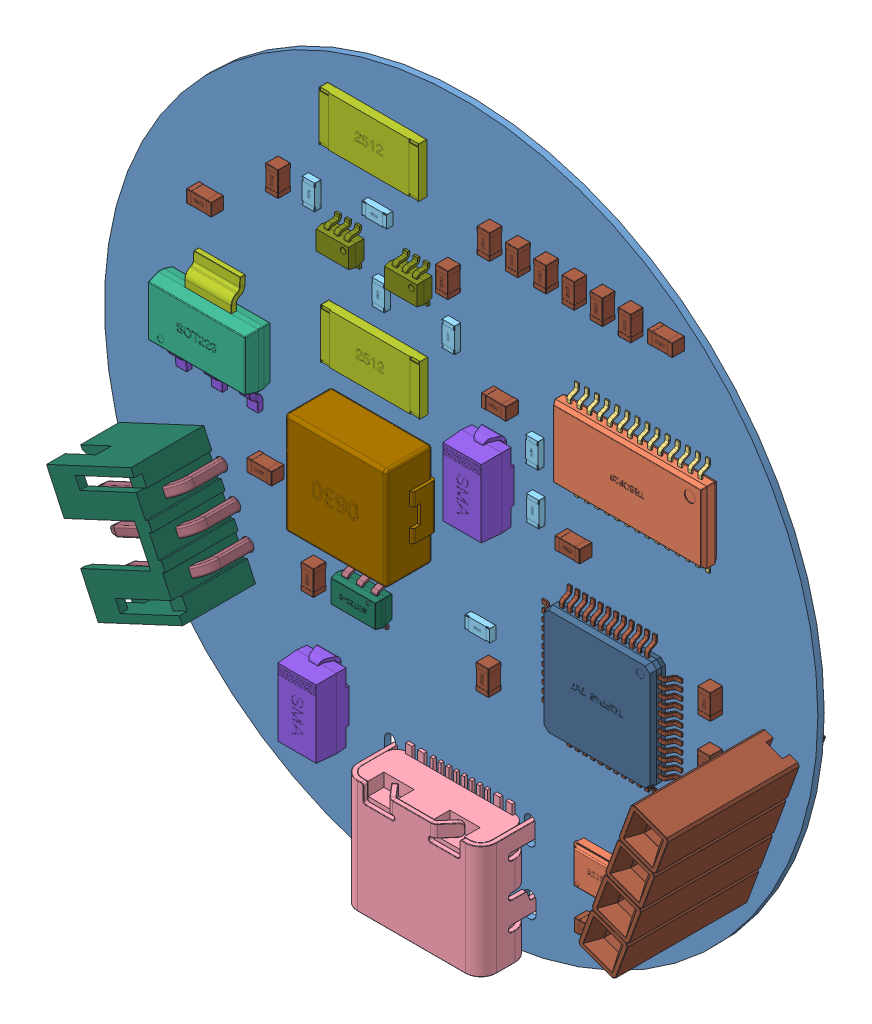
SolidWorks assembly STM32G4_4008_brushless_motor_pcb, configuration 默认. Lengths in mm.
Overall size (46 46 11.81).
338 component instances, 47 part files, 0 mates.
Components (placement in the parent):
- STM32G4_4008_brushless_motor_pcb.step-1: STM32G4_4008_brushless_motor_pcb.step [默认] at origin size (46 46 11.81)
  - Board.step-1: Board.step [默认] at origin size (46 46 0.41)
    - Open CASCADE STEP translator 6.8 1.1.1.step-1: Open CASCADE STEP translator 6.8 1.1.1.step [默认] at (0 0 -0.4115) size (46 46 0.41)
  - X1.step-1: X1.step [默认] at origin size (3.2 2.5 0.72)
    - OSC_3225-4.step-1: OSC_3225-4.step [默认] at (100.5332 55.0164 0) size (3.2 2.5 0.72)
      - OSC_3225-4-0.step-1: OSC_3225-4-0.step [默认] at origin size (3.2 2.5 0.72)
      - LOGO_0.15.step-1: LOGO_0.15.step [默认] at (-0.0166 0.0115 -0.003) size (0.45 0.52 0)
  - USB1.step-1: USB1.step [默认] at origin size (8.94 7.9 4.1)
    - USB_Type-C_A.step-1: USB_Type-C_A.step [默认] at (91.2368 50.7239 0) x (-1 0 0) z (0 0 1) size (8.94 7.9 4.1)
      - USB_Type-C_A-1.step-1: USB_Type-C_A-1.step [默认] at origin size (8.94 7.9 4.1)
      - LOGO_0.5.step-1: LOGO_0.5.step [默认] at (0.0308 -0.1109 0.04) size (1.5 1.73 0.01)
  - U7.step-1: U7.step [默认] at origin size (6.5 7.02 1.67)
    - SOT223.step-1: SOT223.step [默认] at (75.7682 73.3044 0) size (6.5 7.02 1.67)
      - SOT223-2.step-1: SOT223-2.step [默认] at origin size (6.5 3.5 1.6)
      - SOT223___-1.step-1: SOT223___-1.step [默认] at (0 1.75 0.725) size (3 1.76 0.92)
      - SOT223___-2.step-1: SOT223___-2.step [默认] at (2.3 -1.75 0.725) x (-1 0 0) z (0 0 1) size (0.71 1.76 0.92)
      - SOT223___-2.step-2: SOT223___-2.step [默认] at (0 -1.75 0.725) x (-1 0 0) z (0 0 1) size (0.71 1.76 0.92)
      - SOT223___-2.step-3: SOT223___-2.step [默认] at (-2.3 -1.75 0.725) x (-1 0 0) z (0 0 1) size (0.71 1.76 0.92)
      - LOGO_0.25.step-1: LOGO_0.25.step [默认] at origin size (0.75 0.87 0.01)
  - U6.step-1: U6.step [默认] at origin size (9 9 1.05)
    - TQFP48_7x7.step-1: TQFP48_7x7.step [默认] at (100.9904 65.4812 0) x (-1 0 0) z (0 0 1) size (9 9 1.05)
      - TQFP48_7x7______.step-1: TQFP48_7x7______.step [默认] at origin size (7 7 1)
      - _____0.25.step-1: _____0.25.step [默认] at (2.75 -3.5 0.55) x (-1 0 0) z (0 0 1) size (0.25 1 0.6)
      - _____0.25.step-2: _____0.25.step [默认] at (2.25 -3.5 0.55) x (-1 0 0) z (0 0 1) size (0.25 1 0.6)
      - _____0.25.step-3: _____0.25.step [默认] at (1.75 -3.5 0.55) x (-1 0 0) z (0 0 1) size (0.25 1 0.6)
      - _____0.25.step-4: _____0.25.step [默认] at (1.25 -3.5 0.55) x (-1 0 0) z (0 0 1) size (0.25 1 0.6)
      - _____0.25.step-5: _____0.25.step [默认] at (0.75 -3.5 0.55) x (-1 0 0) z (0 0 1) size (0.25 1 0.6)
      - _____0.25.step-6: _____0.25.step [默认] at (0.25 -3.5 0.55) x (-1 0 0) z (0 0 1) size (0.25 1 0.6)
      - _____0.25.step-7: _____0.25.step [默认] at (-0.25 -3.5 0.55) x (-1 0 0) z (0 0 1) size (0.25 1 0.6)
      - _____0.25.step-8: _____0.25.step [默认] at (-0.75 -3.5 0.55) x (-1 0 0) z (0 0 1) size (0.25 1 0.6)
      - _____0.25.step-9: _____0.25.step [默认] at (-1.25 -3.5 0.55) x (-1 0 0) z (0 0 1) size (0.25 1 0.6)
      - _____0.25.step-10: _____0.25.step [默认] at (-1.75 -3.5 0.55) x (-1 0 0) z (0 0 1) size (0.25 1 0.6)
      - _____0.25.step-11: _____0.25.step [默认] at (-2.25 -3.5 0.55) x (-1 0 0) z (0 0 1) size (0.25 1 0.6)
      - _____0.25.step-12: _____0.25.step [默认] at (-2.75 -3.5 0.55) x (-1 0 0) z (0 0 1) size (0.25 1 0.6)
      - _____0.25.step-13: _____0.25.step [默认] at (3.5 2.75 0.55) x (0 -1 0) z (0 0 1) size (0.25 1 0.6)
      - _____0.25.step-14: _____0.25.step [默认] at (-2.75 3.5 0.55) size (0.25 1 0.6)
      - _____0.25.step-15: _____0.25.step [默认] at (-3.5 -2.75 0.55) x (0 1 0) z (0 0 1) size (0.25 1 0.6)
      - _____0.25.step-16: _____0.25.step [默认] at (3.5 2.25 0.55) x (0 -1 0) z (0 0 1) size (0.25 1 0.6)
      - _____0.25.step-17: _____0.25.step [默认] at (-2.25 3.5 0.55) size (0.25 1 0.6)
      - _____0.25.step-18: _____0.25.step [默认] at (-3.5 -2.25 0.55) x (0 1 0) z (0 0 1) size (0.25 1 0.6)
      - _____0.25.step-19: _____0.25.step [默认] at (3.5 1.75 0.55) x (0 -1 0) z (0 0 1) size (0.25 1 0.6)
      - _____0.25.step-20: _____0.25.step [默认] at (-1.75 3.5 0.55) size (0.25 1 0.6)
      - _____0.25.step-21: _____0.25.step [默认] at (-3.5 -1.75 0.55) x (0 1 0) z (0 0 1) size (0.25 1 0.6)
      - _____0.25.step-22: _____0.25.step [默认] at (3.5 1.25 0.55) x (0 -1 0) z (0 0 1) size (0.25 1 0.6)
      - _____0.25.step-23: _____0.25.step [默认] at (-1.25 3.5 0.55) size (0.25 1 0.6)
      - _____0.25.step-24: _____0.25.step [默认] at (-3.5 -1.25 0.55) x (0 1 0) z (0 0 1) size (0.25 1 0.6)
      - _____0.25.step-25: _____0.25.step [默认] at (3.5 0.75 0.55) x (0 -1 0) z (0 0 1) size (0.25 1 0.6)
      - _____0.25.step-26: _____0.25.step [默认] at (-0.75 3.5 0.55) size (0.25 1 0.6)
      - _____0.25.step-27: _____0.25.step [默认] at (-3.5 -0.75 0.55) x (0 1 0) z (0 0 1) size (0.25 1 0.6)
      - _____0.25.step-28: _____0.25.step [默认] at (3.5 0.25 0.55) x (0 -1 0) z (0 0 1) size (0.25 1 0.6)
      - _____0.25.step-29: _____0.25.step [默认] at (-0.25 3.5 0.55) size (0.25 1 0.6)
      - _____0.25.step-30: _____0.25.step [默认] at (-3.5 -0.25 0.55) x (0 1 0) z (0 0 1) size (0.25 1 0.6)
      - _____0.25.step-31: _____0.25.step [默认] at (3.5 -0.25 0.55) x (0 -1 0) z (0 0 1) size (0.25 1 0.6)
      - _____0.25.step-32: _____0.25.step [默认] at (0.25 3.5 0.55) size (0.25 1 0.6)
      - _____0.25.step-33: _____0.25.step [默认] at (-3.5 0.25 0.55) x (0 1 0) z (0 0 1) size (0.25 1 0.6)
      - _____0.25.step-34: _____0.25.step [默认] at (3.5 -0.75 0.55) x (0 -1 0) z (0 0 1) size (0.25 1 0.6)
      - _____0.25.step-35: _____0.25.step [默认] at (0.75 3.5 0.55) size (0.25 1 0.6)
      - _____0.25.step-36: _____0.25.step [默认] at (-3.5 0.75 0.55) x (0 1 0) z (0 0 1) size (0.25 1 0.6)
      - _____0.25.step-37: _____0.25.step [默认] at (3.5 -1.25 0.55) x (0 -1 0) z (0 0 1) size (0.25 1 0.6)
      - _____0.25.step-38: _____0.25.step [默认] at (1.25 3.5 0.55) size (0.25 1 0.6)
      - _____0.25.step-39: _____0.25.step [默认] at (-3.5 1.25 0.55) x (0 1 0) z (0 0 1) size (0.25 1 0.6)
      - _____0.25.step-40: _____0.25.step [默认] at (3.5 -1.75 0.55) x (0 -1 0) z (0 0 1) size (0.25 1 0.6)
      - _____0.25.step-41: _____0.25.step [默认] at (1.75 3.5 0.55) size (0.25 1 0.6)
      - _____0.25.step-42: _____0.25.step [默认] at (-3.5 1.75 0.55) x (0 1 0) z (0 0 1) size (0.25 1 0.6)
      - _____0.25.step-43: _____0.25.step [默认] at (3.5 -2.25 0.55) x (0 -1 0) z (0 0 1) size (0.25 1 0.6)
      - _____0.25.step-44: _____0.25.step [默认] at (2.25 3.5 0.55) size (0.25 1 0.6)
      - _____0.25.step-45: _____0.25.step [默认] at (-3.5 2.25 0.55) x (0 1 0) z (0 0 1) size (0.25 1 0.6)
      - _____0.25.step-46: _____0.25.step [默认] at (3.5 -2.75 0.55) x (0 -1 0) z (0 0 1) size (0.25 1 0.6)
      - _____0.25.step-47: _____0.25.step [默认] at (2.75 3.5 0.55) size (0.25 1 0.6)
      - _____0.25.step-48: _____0.25.step [默认] at (-3.5 2.75 0.55) x (0 1 0) z (0 0 1) size (0.25 1 0.6)
      - LOGO_0.25-3.step-1: LOGO_0.25-3.step [默认] at (0.012 -0.0139 0.045) size (0.75 0.87 0.01)
  - U5.step-1: U5.step [默认] at origin size (3 2.81 1.18)
    - SOT23-6.step-1: SOT23-6.step [默认] at (85.3693 63.043 0) x (-1 0 0) z (0 0 1) size (3 2.81 1.18)
      - SOT23-5and6_____.step-1: SOT23-5and6_____.step [默认] at (-0.95 -0.8 0.675) x (-1 0 0) z (0 0 1) size (0.4 0.6 0.78)
      - SOT23-5and6_____.step-2: SOT23-5and6_____.step [默认] at (0 -0.8 0.675) x (-1 0 0) z (0 0 1) size (0.4 0.6 0.78)
      - SOT23-5and6_____.step-3: SOT23-5and6_____.step [默认] at (0.95 -0.8 0.675) x (-1 0 0) z (0 0 1) size (0.4 0.6 0.78)
      - SOT23-5and6_____.step-4: SOT23-5and6_____.step [默认] at (-0.95 0.8 0.675) size (0.4 0.6 0.78)
      - SOT23-5and6_____.step-5: SOT23-5and6_____.step [默认] at (0.95 0.8 0.675) size (0.4 0.6 0.78)
      - LOGO_0.15-4.step-1: LOGO_0.15-4.step [默认] at (0 -0.0167 0.0485) x (-1 0 0) z (0 0 -1) size (0.45 0.52 0)
      - SOT23-6-5.step-1: SOT23-6-5.step [默认] at origin size (3 1.6 1.1)
      - SOT23-5and6_____.step-6: SOT23-5and6_____.step [默认] at (0 0.8 0.675) size (0.4 0.6 0.78)
  - U4.step-1: U4.step [默认] at origin size (2.2 2.4 1.1)
    - User_Library-SOT363-2.step-1: User_Library-SOT363-2.step [默认] at (83.9827 82.123 0) x (-1 0 0) z (0 0 1) size (2.2 2.4 1.1)
  - U3.step-1: U3.step [默认] at origin size (2.2 2.4 1.1)
    - User_Library-SOT363-2.step-1: User_Library-SOT363-2.step [默认] at (88.3815 82.2404 0) x (-1 0 0) z (0 0 1) size (2.2 2.4 1.1)
  - U2.step-1: U2.step [默认] at origin size (6.01 5 1.9)
    - SOP8.step-1: SOP8.step [默认] at (91.186 70.612 -0.4115) x (-1 0 0) z (0 0 -1) size (6.01 5 1.9)
      - LOGO_0.25-6.step-1: LOGO_0.25-6.step [默认] at (0.0116 0 0.095) x (0 -1 0) z (0 0 -1) size (0.75 0.87 0.01)
      - SOP8_____.step-1: SOP8_____.step [默认] at origin size (3.6 5 1.8)
      - ____1.8_______.step-1: ____1.8_______.step [默认] at (1.8 1.91 1) x (0 1 0) z (0 0 1) size (0.5 1.2 1.1)
      - ____1.8_______.step-2: ____1.8_______.step [默认] at (1.8 0.64 1) x (0 1 0) z (0 0 1) size (0.5 1.2 1.1)
      - ____1.8_______.step-3: ____1.8_______.step [默认] at (1.8 -0.63 1) x (0 1 0) z (0 0 1) size (0.5 1.2 1.1)
      - ____1.8_______.step-4: ____1.8_______.step [默认] at (1.8 -1.9 1) x (0 1 0) z (0 0 1) size (0.5 1.2 1.1)
      - ____1.8_______.step-5: ____1.8_______.step [默认] at (-1.8 1.91 1) x (0 -1 0) z (0 0 1) size (0.5 1.2 1.1)
      - ____1.8_______.step-6: ____1.8_______.step [默认] at (-1.8 0.64 1) x (0 -1 0) z (0 0 1) size (0.5 1.2 1.1)
      - ____1.8_______.step-7: ____1.8_______.step [默认] at (-1.8 -0.63 1) x (0 -1 0) z (0 0 1) size (0.5 1.2 1.1)
      - ____1.8_______.step-8: ____1.8_______.step [默认] at (-1.8 -1.9 1) x (0 -1 0) z (0 0 1) size (0.5 1.2 1.1)
  - U1.step-1: U1.step [默认] at origin size (9.8 6.4 1.05)
    - TSSOP28.step-1: TSSOP28.step [默认] at (102.9208 78.3336 0) x (0 -1 0) z (0 0 1) size (6.4 9.8 1.05)
      - TSSOP28_____.step-1: TSSOP28_____.step [默认] at origin size (4.6 9.8 1)
      - _____0.9.step-1: _____0.9.step [默认] at (-2.3 4.225 0.53) x (0 -1 0) z (0 0 1) size (0.25 0.9 0.6)
      - _____0.9.step-2: _____0.9.step [默认] at (-2.3 3.575 0.53) x (0 -1 0) z (0 0 1) size (0.25 0.9 0.6)
      - _____0.9.step-3: _____0.9.step [默认] at (-2.3 2.925 0.53) x (0 -1 0) z (0 0 1) size (0.25 0.9 0.6)
      - _____0.9.step-4: _____0.9.step [默认] at (-2.3 2.275 0.53) x (0 -1 0) z (0 0 1) size (0.25 0.9 0.6)
      - _____0.9.step-5: _____0.9.step [默认] at (-2.3 1.625 0.53) x (0 -1 0) z (0 0 1) size (0.25 0.9 0.6)
      - _____0.9.step-6: _____0.9.step [默认] at (-2.3 0.975 0.53) x (0 -1 0) z (0 0 1) size (0.25 0.9 0.6)
      - _____0.9.step-7: _____0.9.step [默认] at (-2.3 0.325 0.53) x (0 -1 0) z (0 0 1) size (0.25 0.9 0.6)
      - _____0.9.step-8: _____0.9.step [默认] at (-2.3 -0.325 0.53) x (0 -1 0) z (0 0 1) size (0.25 0.9 0.6)
      - _____0.9.step-9: _____0.9.step [默认] at (-2.3 -0.975 0.53) x (0 -1 0) z (0 0 1) size (0.25 0.9 0.6)
      - _____0.9.step-10: _____0.9.step [默认] at (-2.3 -1.625 0.53) x (0 -1 0) z (0 0 1) size (0.25 0.9 0.6)
      - _____0.9.step-11: _____0.9.step [默认] at (-2.3 -2.275 0.53) x (0 -1 0) z (0 0 1) size (0.25 0.9 0.6)
      - _____0.9.step-12: _____0.9.step [默认] at (-2.3 -2.925 0.53) x (0 -1 0) z (0 0 1) size (0.25 0.9 0.6)
      - _____0.9.step-13: _____0.9.step [默认] at (-2.3 -3.575 0.53) x (0 -1 0) z (0 0 1) size (0.25 0.9 0.6)
      - _____0.9.step-14: _____0.9.step [默认] at (-2.3 -4.225 0.53) x (0 -1 0) z (0 0 1) size (0.25 0.9 0.6)
      - _____0.9.step-15: _____0.9.step [默认] at (2.3 4.225 0.53) x (0 1 0) z (0 0 1) size (0.25 0.9 0.6)
      - _____0.9.step-16: _____0.9.step [默认] at (2.3 3.575 0.53) x (0 1 0) z (0 0 1) size (0.25 0.9 0.6)
      - _____0.9.step-17: _____0.9.step [默认] at (2.3 2.925 0.53) x (0 1 0) z (0 0 1) size (0.25 0.9 0.6)
      - _____0.9.step-18: _____0.9.step [默认] at (2.3 2.275 0.53) x (0 1 0) z (0 0 1) size (0.25 0.9 0.6)
      - _____0.9.step-19: _____0.9.step [默认] at (2.3 1.625 0.53) x (0 1 0) z (0 0 1) size (0.25 0.9 0.6)
      - _____0.9.step-20: _____0.9.step [默认] at (2.3 0.975 0.53) x (0 1 0) z (0 0 1) size (0.25 0.9 0.6)
      - _____0.9.step-21: _____0.9.step [默认] at (2.3 0.325 0.53) x (0 1 0) z (0 0 1) size (0.25 0.9 0.6)
      - _____0.9.step-22: _____0.9.step [默认] at (2.3 -0.325 0.53) x (0 1 0) z (0 0 1) size (0.25 0.9 0.6)
      - _____0.9.step-23: _____0.9.step [默认] at (2.3 -0.975 0.53) x (0 1 0) z (0 0 1) size (0.25 0.9 0.6)
      - _____0.9.step-24: _____0.9.step [默认] at (2.3 -1.625 0.53) x (0 1 0) z (0 0 1) size (0.25 0.9 0.6)
      - _____0.9.step-25: _____0.9.step [默认] at (2.3 -2.275 0.53) x (0 1 0) z (0 0 1) size (0.25 0.9 0.6)
      - _____0.9.step-26: _____0.9.step [默认] at (2.3 -2.925 0.53) x (0 1 0) z (0 0 1) size (0.25 0.9 0.6)
      - _____0.9.step-27: _____0.9.step [默认] at (2.3 -3.575 0.53) x (0 1 0) z (0 0 1) size (0.25 0.9 0.6)
      - _____0.9.step-28: _____0.9.step [默认] at (2.3 -4.225 0.53) x (0 1 0) z (0 0 1) size (0.25 0.9 0.6)
      - LOGO_0.25-7.step-1: LOGO_0.25-7.step [默认] at (0 0.1751 0.025) size (0.75 0.87 0.01)
  - R16.step-1: R16.step [默认] at origin size (1.6 0.8 0.41)
    - R_0603-HP.step-1: R_0603-HP.step [默认] at (103.3526 58.9789 -0.4115) x (-1 0 0) z (0 0 -1) size (1.6 0.8 0.4)
      - R_0603.step-1: R_0603.step [默认] at origin size (1.6 0.8 0.4)
      - LOGO_.step-1: LOGO_.step [默认] at (0.0001 0.0322 -0.002) x (-1 0 0) z (0 0 -1) size (0.6 0.69 0)
  - R15.step-1: R15.step [默认] at origin size (0.8 1.6 0.4)
    - R_0603-HP.step-1: R_0603-HP.step [默认] at (96.1897 73.2536 0) x (0 1 0) z (0 0 1) size (1.6 0.8 0.4)
      - R_0603.step-1: R_0603.step [默认] at origin size (1.6 0.8 0.4)
      - LOGO_.step-1: LOGO_.step [默认] at (0.0001 0.0322 -0.002) x (-1 0 0) z (0 0 -1) size (0.6 0.69 0)
  - R14.step-1: R14.step [默认] at origin size (0.8 1.6 0.4)
    - R_0603-HP.step-1: R_0603-HP.step [默认] at (96.1389 76.5048 0) x (0 1 0) z (0 0 1) size (1.6 0.8 0.4)
      - R_0603.step-1: R_0603.step [默认] at origin size (1.6 0.8 0.4)
      - LOGO_.step-1: LOGO_.step [默认] at (0.0001 0.0322 -0.002) x (-1 0 0) z (0 0 -1) size (0.6 0.69 0)
  - R13.step-1: R13.step [默认] at origin size (1.6 0.8 0.4)
    - R_0603-HP.step-1: R_0603-HP.step [默认] at (92.6234 64.8969 0) x (-1 0 0) z (0 0 1) size (1.6 0.8 0.4)
      - R_0603.step-1: R_0603.step [默认] at origin size (1.6 0.8 0.4)
      - LOGO_.step-1: LOGO_.step [默认] at (0.0001 0.0322 -0.002) x (-1 0 0) z (0 0 -1) size (0.6 0.69 0)
  - R12.step-1: R12.step [默认] at origin size (0.8 1.6 0.41)
    - R_0603-HP.step-1: R_0603-HP.step [默认] at (97.2313 60.8688 -0.4115) x (0 1 0) z (0 0 -1) size (1.6 0.8 0.4)
      - R_0603.step-1: R_0603.step [默认] at origin size (1.6 0.8 0.4)
      - LOGO_.step-1: LOGO_.step [默认] at (0.0001 0.0322 -0.002) x (-1 0 0) z (0 0 -1) size (0.6 0.69 0)
  - R11.step-1: R11.step [默认] at origin size (0.8 1.6 0.41)
    - R_0603-HP.step-1: R_0603-HP.step [默认] at (95.0215 60.8688 -0.4115) x (0 1 0) z (0 0 -1) size (1.6 0.8 0.4)
      - R_0603.step-1: R_0603.step [默认] at origin size (1.6 0.8 0.4)
      - LOGO_.step-1: LOGO_.step [默认] at (0.0001 0.0322 -0.002) x (-1 0 0) z (0 0 -1) size (0.6 0.69 0)
  - R10.step-1: R10.step [默认] at origin size (0.8 1.6 0.41)
    - R_0603-HP.step-1: R_0603-HP.step [默认] at (92.8117 60.8688 -0.4115) x (0 1 0) z (0 0 -1) size (1.6 0.8 0.4)
      - R_0603.step-1: R_0603.step [默认] at origin size (1.6 0.8 0.4)
      - LOGO_.step-1: LOGO_.step [默认] at (0.0001 0.0322 -0.002) x (-1 0 0) z (0 0 -1) size (0.6 0.69 0)
  - R9.step-1: R9.step [默认] at origin size (1.6 0.8 0.4)
    - R_0603-HP.step-1: R_0603-HP.step [默认] at (85.979 84.6835 0) x (-1 0 0) z (0 0 1) size (1.6 0.8 0.4)
      - R_0603.step-1: R_0603.step [默认] at origin size (1.6 0.8 0.4)
      - LOGO_.step-1: LOGO_.step [默认] at (0.0001 0.0322 -0.002) x (-1 0 0) z (0 0 -1) size (0.6 0.69 0)
  - R8.step-1: R8.step [默认] at origin size (6.4 3.2 0.57)
    - R_2512-HP.step-1: R_2512-HP.step [默认] at (85.7758 88.5953 0) x (1 0 0) z (0 0 1) size (6.4 3.2 0.57)
      - R_2512.step-1: R_2512.step [默认] at origin size (6.4 3.2 0.55)
      - LOGO_-8.step-1: LOGO_-8.step [默认] at (-0.005 0.1842 -0.008) x (-1 0 0) z (0 0 -1) size (2.4 2.77 0.02)
  - R7.step-1: R7.step [默认] at origin size (0.8 1.6 0.4)
    - R_0603-HP.step-1: R_0603-HP.step [默认] at (81.7373 83.7334 0) x (0 -1 0) z (0 0 1) size (1.6 0.8 0.4)
      - R_0603.step-1: R_0603.step [默认] at origin size (1.6 0.8 0.4)
      - LOGO_.step-1: LOGO_.step [默认] at (0.0001 0.0322 -0.002) x (-1 0 0) z (0 0 -1) size (0.6 0.69 0)
  - R6.step-1: R6.step [默认] at origin size (0.8 1.6 0.4)
    - R_0603-HP.step-1: R_0603-HP.step [默认] at (90.7541 80.264 0) x (0 1 0) z (0 0 1) size (1.6 0.8 0.4)
      - R_0603.step-1: R_0603.step [默认] at origin size (1.6 0.8 0.4)
      - LOGO_.step-1: LOGO_.step [默认] at (0.0001 0.0322 -0.002) x (-1 0 0) z (0 0 -1) size (0.6 0.69 0)
  - R5.step-1: R5.step [默认] at origin size (1.6 0.8 0.41)
    - R_0603-HP.step-1: R_0603-HP.step [默认] at (89.1898 66.2179 -0.4115) x (-1 0 0) z (0 0 -1) size (1.6 0.8 0.4)
      - R_0603.step-1: R_0603.step [默认] at origin size (1.6 0.8 0.4)
      - LOGO_.step-1: LOGO_.step [默认] at (0.0001 0.0322 -0.002) x (-1 0 0) z (0 0 -1) size (0.6 0.69 0)
  - R4.step-1: R4.step [默认] at origin size (6.4 3.2 0.57)
    - R_2512-HP.step-1: R_2512-HP.step [默认] at (85.8521 76.4795 0) x (1 0 0) z (0 0 1) size (6.4 3.2 0.57)
      - R_2512.step-1: R_2512.step [默认] at origin size (6.4 3.2 0.55)
      - LOGO_-8.step-1: LOGO_-8.step [默认] at (-0.005 0.1842 -0.008) x (-1 0 0) z (0 0 -1) size (2.4 2.77 0.02)
  - R3.step-1: R3.step [默认] at origin size (0.8 1.6 0.4)
    - R_0603-HP.step-1: R_0603-HP.step [默认] at (86.2329 80.3402 0) x (0 1 0) z (0 0 1) size (1.6 0.8 0.4)
      - R_0603.step-1: R_0603.step [默认] at origin size (1.6 0.8 0.4)
      - LOGO_.step-1: LOGO_.step [默认] at (0.0001 0.0322 -0.002) x (-1 0 0) z (0 0 -1) size (0.6 0.69 0)
  - R2.step-1: R2.step [默认] at origin size (0.8 1.6 0.41)
    - R_0603-HP.step-1: R_0603-HP.step [默认] at (84.5567 72.0956 -0.4115) x (0 1 0) z (0 0 -1) size (1.6 0.8 0.4)
      - R_0603.step-1: R_0603.step [默认] at origin size (1.6 0.8 0.4)
      - LOGO_.step-1: LOGO_.step [默认] at (0.0001 0.0322 -0.002) x (-1 0 0) z (0 0 -1) size (0.6 0.69 0)
  - R1.step-1: R1.step [默认] at origin size (0.8 1.6 0.41)
    - R_0603-HP.step-1: R_0603-HP.step [默认] at (84.5565 68.5695 -0.4115) x (0 -1 0) z (0 0 -1) size (1.6 0.8 0.4)
      - R_0603.step-1: R_0603.step [默认] at origin size (1.6 0.8 0.4)
      - LOGO_.step-1: LOGO_.step [默认] at (0.0001 0.0322 -0.002) x (-1 0 0) z (0 0 -1) size (0.6 0.69 0)
  - L1.step-1: L1.step [默认] at origin size (6.95 6.6 3.03)
    - SMD-0630.step-1: SMD-0630.step [默认] at (86.1314 70.104 0) x (-1 0 0) z (0 0 1) size (6.95 6.6 3.03)
      - SMD-0630-9.step-1: SMD-0630-9.step [默认] at origin size (6.95 6.6 3.03)
      - LOGO_0.5-10.step-1: LOGO_0.5-10.step [默认] at (0 0.0017 0.04) size (1.5 1.73 0.01)
  - J3.step-1: J3.step [默认] at origin size (5.86 10.42 11.5)
    - HDR2.54-1P_M.step-1: HDR2.54-1P_M.step [默认] at (109.7 61.824 0) x (0.34202 0.939693 0) z (0 0 1) size (2.54 2.54 11.5)
      - HDR2.54-1P_M-11.step-1: HDR2.54-1P_M-11.step [默认] at origin size (2.54 2.54 11.5)
      - LOGO_-12.step-1: LOGO_-12.step [默认] at (0 0.9721 0.0285) x (-1 0 0) z (0 0 -1) size (0.45 0.52 0)
    - HDR2.54-1P_M.step-2: HDR2.54-1P_M.step [默认] at (108.8313 59.4372 0) x (0.34202 0.939693 0) z (0 0 1) size (2.54 2.54 11.5)
      - HDR2.54-1P_M-11.step-1: HDR2.54-1P_M-11.step [默认] at origin size (2.54 2.54 11.5)
      - LOGO_-12.step-1: LOGO_-12.step [默认] at (0 0.9721 0.0285) x (-1 0 0) z (0 0 -1) size (0.45 0.52 0)
    - HDR2.54-1P_M.step-3: HDR2.54-1P_M.step [默认] at (111.4375 66.5976 0) x (0.34202 0.939693 0) z (0 0 1) size (2.54 2.54 11.5)
      - HDR2.54-1P_M-11.step-1: HDR2.54-1P_M-11.step [默认] at origin size (2.54 2.54 11.5)
      - LOGO_-12.step-1: LOGO_-12.step [默认] at (0 0.9721 0.0285) x (-1 0 0) z (0 0 -1) size (0.45 0.52 0)
    - HDR2.54-1P_M.step-4: HDR2.54-1P_M.step [默认] at (110.5688 64.2108 0) x (0.34202 0.939693 0) z (0 0 1) size (2.54 2.54 11.5)
      - HDR2.54-1P_M-11.step-1: HDR2.54-1P_M-11.step [默认] at origin size (2.54 2.54 11.5)
      - LOGO_-12.step-1: LOGO_-12.step [默认] at (0 0.9721 0.0285) x (-1 0 0) z (0 0 -1) size (0.45 0.52 0)
  - J2.step-1: J2.step [默认] at origin size (9.32 9.95 7.4)
    - PH2.0-WI-3P.step-1: PH2.0-WI-3P.step [默认] at (76.581 63.627 0) x (0.422618 -0.906308 0) z (0 0 1) size (7.9 6.6 7.4)
      - PH2.0-WI-____.step-1: PH2.0-WI-____.step [默认] at (-2 0 0.05) size (0.6 5.5 6)
      - PH2.0-WI-____.step-2: PH2.0-WI-____.step [默认] at (0 0 0.05) size (0.6 5.5 6)
      - LOGO_0.25-13.step-1: LOGO_0.25-13.step [默认] at (-0.0263 -2.2762 0.045) size (0.75 0.87 0.01)
      - PH2.0-WI-____.step-3: PH2.0-WI-____.step [默认] at (2 0 0.05) size (0.6 5.5 6)
      - PH2.0-WI-3P-14.step-1: PH2.0-WI-3P-14.step [默认] at origin size (7.9 6 4.7)
  - J1.step-1: J1.step [默认] at origin size (5 4.95 2.9)
    - 3D_Model.step-1: 3D_Model.step [默认] at (79.8815 81.6977 -0.4115) x (-1 0 0) z (0 -1 0) size (5 2.9 4.95)
      - SH_1_0-LT-3P_ASM_1_AF0_ASM.step-1: SH_1_0-LT-3P_ASM_1_AF0_ASM.step [默认] at origin size (5 2.9 4.95)
        - ID20001_ASM_1_AF0_ASM_1_AF0_ASM.step-1: ID20001_ASM_1_AF0_ASM_1_AF0_ASM.step [默认] at origin size (5 2.9 4.95)
          - 3DID1_AF00001_ASM_1_AF0_ASM_1_ASM.step-1: 3DID1_AF00001_ASM_1_AF0_ASM_1_ASM.step [默认] at origin size (3.6 2.9 4.95)
            - LPATTERN3_11__1_AF0_1_1_1_2.step-1: LPATTERN3_11__1_AF0_1_1_1_2.step [默认] at origin size (0.2 2.4 1.2)
            - LPATTERN3_7__1_3_1.step-1: LPATTERN3_7__1_3_1.step [默认] at origin size (0.2 2.4 1.2)
            - LPATTERN3_2__1_3_1.step-1: LPATTERN3_2__1_3_1.step [默认] at origin size (0.2 2.4 1.2)
            - LPATTERN3_6__1_AF0_3_1.step-1: LPATTERN3_6__1_AF0_3_1.step [默认] at origin size (0.2 2.4 1.2)
            - EXTRUDE8_1_1_1.step-1: EXTRUDE8_1_1_1.step [默认] at origin size (0.3 1.25 1.5)
            - PIN_1_MARK_1_AF0_3_AF0_1.step-1: PIN_1_MARK_1_AF0_3_AF0_1.step [默认] at origin size (3.6 2.8 4.25)
            - LPATTERN3_3__1_1_1.step-1: LPATTERN3_3__1_1_1.step [默认] at origin size (0.2 2.4 1.2)
            - LPATTERN3_1__1_AF0_3_1.step-1: LPATTERN3_1__1_AF0_3_1.step [默认] at origin size (0.2 2.4 1.2)
          - SH1_0-2L_ASM_1_AF0_ASM_1_AF0_ASM.step-1: SH1_0-2L_ASM_1_AF0_ASM_1_AF0_ASM.step [默认] at (-3 0 0) size (1.4 2.9 4.25)
            - ID0001_ASM_1_ASM_1_AF0_ASM_1_AF0_ASM.step-1: ID0001_ASM_1_ASM_1_AF0_ASM_1_AF0_ASM.step [默认] at origin size (1.4 2.9 4.25)
              - EXTRUDE7_1_1_1_1_AF0.step-1: EXTRUDE7_1_1_1_1_AF0.step [默认] at origin size (0.3 1.25 1.5)
              - PIN_1_MARK_AF0_1_1_AF0_1.step-1: PIN_1_MARK_AF0_1_1_AF0_1.step [默认] at origin size (1.4 2.8 4.25)
  - D2.step-1: D2.step [默认] at origin size (2.6 5.12 2.11)
    - SMA.step-1: SMA.step [默认] at (93.3957 73.7591 0.05) x (0 -1 0) z (0 0 1) size (5.12 2.6 2.11)
      - SMA-15.step-1: SMA-15.step [默认] at origin size (5.12 2.6 2.1)
      - LOGO______.__.step-1: LOGO______.__.step [默认] at (0.0018 0.0048 -0.003) x (-1 0 0) z (0 0 -1) size (0.9 1.04 0.01)
  - D1.step-1: D1.step [默认] at origin size (2.6 5.12 2.11)
    - SMA.step-1: SMA.step [默认] at (82.7531 56.1315 0.05) x (0 -1 0) z (0 0 1) size (5.12 2.6 2.11)
      - SMA-15.step-1: SMA-15.step [默认] at origin size (5.12 2.6 2.1)
      - LOGO______.__.step-1: LOGO______.__.step [默认] at (0.0018 0.0048 -0.003) x (-1 0 0) z (0 0 -1) size (0.9 1.04 0.01)
  - C24.step-1: C24.step [默认] at origin size (1.6 0.82 0.82)
    - C_0603.step-1: C_0603.step [默认] at (78.9686 67.0306 0) x (1 0 0) z (0 0 1) size (1.6 0.82 0.82)
      - LOGO_-16.step-1: LOGO_-16.step [默认] at (0 0.0171 -0.0006) x (-1 0 0) z (0 0 -1) size (0.51 0.59 0)
      - C_0603-17.step-1: C_0603-17.step [默认] at origin size (1.6 0.82 0.82)
  - C23.step-1: C23.step [默认] at origin size (1.6 0.82 0.82)
    - C_0603.step-1: C_0603.step [默认] at (75.0824 80.1116 0) x (1 0 0) z (0 0 1) size (1.6 0.82 0.82)
      - LOGO_-16.step-1: LOGO_-16.step [默认] at (0 0.0171 -0.0006) x (-1 0 0) z (0 0 -1) size (0.51 0.59 0)
      - C_0603-17.step-1: C_0603-17.step [默认] at origin size (1.6 0.82 0.82)
  - C22.step-1: C22.step [默认] at origin size (1.6 0.82 0.82)
    - C_0603.step-1: C_0603.step [默认] at (103.3526 60.5282 -0.4115) x (1 0 0) z (0 0 -1) size (1.6 0.82 0.82)
      - LOGO_-16.step-1: LOGO_-16.step [默认] at (0 0.0171 -0.0006) x (-1 0 0) z (0 0 -1) size (0.51 0.59 0)
      - C_0603-17.step-1: C_0603-17.step [默认] at origin size (1.6 0.82 0.82)
  - C21.step-1: C21.step [默认] at origin size (0.82 1.6 0.82)
    - C_0603.step-1: C_0603.step [默认] at (82.0674 62.5602 0) x (0 1 0) z (0 0 1) size (1.6 0.82 0.82)
      - LOGO_-16.step-1: LOGO_-16.step [默认] at (0 0.0171 -0.0006) x (-1 0 0) z (0 0 -1) size (0.51 0.59 0)
      - C_0603-17.step-1: C_0603-17.step [默认] at origin size (1.6 0.82 0.82)
  - C20.step-1: C20.step [默认] at origin size (0.82 1.6 0.82)
    - C_0603.step-1: C_0603.step [默认] at (103.632 53.7568 0) x (0 -1 0) z (0 0 1) size (1.6 0.82 0.82)
      - LOGO_-16.step-1: LOGO_-16.step [默认] at (0 0.0171 -0.0006) x (-1 0 0) z (0 0 -1) size (0.51 0.59 0)
      - C_0603-17.step-1: C_0603-17.step [默认] at origin size (1.6 0.82 0.82)
  - C19.step-1: C19.step [默认] at origin size (1.6 0.82 0.82)
    - C_0603.step-1: C_0603.step [默认] at (94.0816 78.2066 0) x (1 0 0) z (0 0 1) size (1.6 0.82 0.82)
      - LOGO_-16.step-1: LOGO_-16.step [默认] at (0 0.0171 -0.0006) x (-1 0 0) z (0 0 -1) size (0.51 0.59 0)
      - C_0603-17.step-1: C_0603-17.step [默认] at origin size (1.6 0.82 0.82)
  - C18.step-1: C18.step [默认] at origin size (0.82 1.6 0.82)
    - C_0603.step-1: C_0603.step [默认] at (107.6452 68.4276 0) x (0 -1 0) z (0 0 1) size (1.6 0.82 0.82)
      - LOGO_-16.step-1: LOGO_-16.step [默认] at (0 0.0171 -0.0006) x (-1 0 0) z (0 0 -1) size (0.51 0.59 0)
      - C_0603-17.step-1: C_0603-17.step [默认] at origin size (1.6 0.82 0.82)
  - C17.step-1: C17.step [默认] at origin size (0.82 1.6 0.82)
    - C_0603.step-1: C_0603.step [默认] at (93.345 62.611 0) x (0 1 0) z (0 0 1) size (1.6 0.82 0.82)
      - LOGO_-16.step-1: LOGO_-16.step [默认] at (0 0.0171 -0.0006) x (-1 0 0) z (0 0 -1) size (0.51 0.59 0)
      - C_0603-17.step-1: C_0603-17.step [默认] at origin size (1.6 0.82 0.82)
  - C16.step-1: C16.step [默认] at origin size (0.82 1.6 0.82)
    - C_0603.step-1: C_0603.step [默认] at (107.6198 64.8866 0) x (0 -1 0) z (0 0 1) size (1.6 0.82 0.82)
      - LOGO_-16.step-1: LOGO_-16.step [默认] at (0 0.0171 -0.0006) x (-1 0 0) z (0 0 -1) size (0.51 0.59 0)
      - C_0603-17.step-1: C_0603-17.step [默认] at origin size (1.6 0.82 0.82)
  - C15.step-1: C15.step [默认] at origin size (1.6 0.82 0.82)
    - C_0603.step-1: C_0603.step [默认] at (98.8314 72.6186 0) x (1 0 0) z (0 0 1) size (1.6 0.82 0.82)
      - LOGO_-16.step-1: LOGO_-16.step [默认] at (0 0.0171 -0.0006) x (-1 0 0) z (0 0 -1) size (0.51 0.59 0)
      - C_0603-17.step-1: C_0603-17.step [默认] at origin size (1.6 0.82 0.82)
  - C14.step-1: C14.step [默认] at origin size (1.6 0.82 0.82)
    - C_0603.step-1: C_0603.step [默认] at (100.0864 51.9176 0) x (1 0 0) z (0 0 1) size (1.6 0.82 0.82)
      - LOGO_-16.step-1: LOGO_-16.step [默认] at (0 0.0171 -0.0006) x (-1 0 0) z (0 0 -1) size (0.51 0.59 0)
      - C_0603-17.step-1: C_0603-17.step [默认] at origin size (1.6 0.82 0.82)
  - C13.step-1: C13.step [默认] at origin size (0.82 1.6 0.82)
    - C_0603.step-1: C_0603.step [默认] at (79.7814 83.693 0) x (0 1 0) z (0 0 1) size (1.6 0.82 0.82)
      - LOGO_-16.step-1: LOGO_-16.step [默认] at (0 0.0171 -0.0006) x (-1 0 0) z (0 0 -1) size (0.51 0.59 0)
      - C_0603-17.step-1: C_0603-17.step [默认] at origin size (1.6 0.82 0.82)
  - C12.step-1: C12.step [默认] at origin size (1.6 0.82 0.82)
    - C_0603.step-1: C_0603.step [默认] at (101.9914 72.6186 -0.4115) x (1 0 0) z (0 0 -1) size (1.6 0.82 0.82)
      - LOGO_-16.step-1: LOGO_-16.step [默认] at (0 0.0171 -0.0006) x (-1 0 0) z (0 0 -1) size (0.51 0.59 0)
      - C_0603-17.step-1: C_0603-17.step [默认] at origin size (1.6 0.82 0.82)
  - C11.step-1: C11.step [默认] at origin size (0.82 1.6 0.82)
    - C_0603.step-1: C_0603.step [默认] at (100.6958 86.995 0) x (0 1 0) z (0 0 1) size (1.6 0.82 0.82)
      - LOGO_-16.step-1: LOGO_-16.step [默认] at (0 0.0171 -0.0006) x (-1 0 0) z (0 0 -1) size (0.51 0.59 0)
      - C_0603-17.step-1: C_0603-17.step [默认] at origin size (1.6 0.82 0.82)
  - C10.step-1: C10.step [默认] at origin size (0.82 1.6 0.82)
    - C_0603.step-1: C_0603.step [默认] at (93.4212 86.995 0) x (0 1 0) z (0 0 1) size (1.6 0.82 0.82)
      - LOGO_-16.step-1: LOGO_-16.step [默认] at (0 0.0171 -0.0006) x (-1 0 0) z (0 0 -1) size (0.51 0.59 0)
      - C_0603-17.step-1: C_0603-17.step [默认] at origin size (1.6 0.82 0.82)
  - C9.step-1: C9.step [默认] at origin size (0.82 1.6 0.82)
    - C_0603.step-1: C_0603.step [默认] at (95.2399 86.995 0) x (0 1 0) z (0 0 1) size (1.6 0.82 0.82)
      - LOGO_-16.step-1: LOGO_-16.step [默认] at (0 0.0171 -0.0006) x (-1 0 0) z (0 0 -1) size (0.51 0.59 0)
      - C_0603-17.step-1: C_0603-17.step [默认] at origin size (1.6 0.82 0.82)
  - C8.step-1: C8.step [默认] at origin size (0.82 1.6 0.82)
    - C_0603.step-1: C_0603.step [默认] at (97.0585 86.995 0) x (0 1 0) z (0 0 1) size (1.6 0.82 0.82)
      - LOGO_-16.step-1: LOGO_-16.step [默认] at (0 0.0171 -0.0006) x (-1 0 0) z (0 0 -1) size (0.51 0.59 0)
      - C_0603-17.step-1: C_0603-17.step [默认] at origin size (1.6 0.82 0.82)
  - C7.step-1: C7.step [默认] at origin size (0.82 1.6 0.82)
    - C_0603.step-1: C_0603.step [默认] at (98.8771 86.995 0) x (0 1 0) z (0 0 1) size (1.6 0.82 0.82)
      - LOGO_-16.step-1: LOGO_-16.step [默认] at (0 0.0171 -0.0006) x (-1 0 0) z (0 0 -1) size (0.51 0.59 0)
      - C_0603-17.step-1: C_0603-17.step [默认] at origin size (1.6 0.82 0.82)
  - C6.step-1: C6.step [默认] at origin size (0.82 1.6 0.82)
    - C_0603.step-1: C_0603.step [默认] at (90.7288 83.5152 0) x (0 1 0) z (0 0 1) size (1.6 0.82 0.82)
      - LOGO_-16.step-1: LOGO_-16.step [默认] at (0 0.0171 -0.0006) x (-1 0 0) z (0 0 -1) size (0.51 0.59 0)
      - C_0603-17.step-1: C_0603-17.step [默认] at origin size (1.6 0.82 0.82)
  - C5.step-1: C5.step [默认] at origin size (0.82 1.6 0.82)
    - C_0603.step-1: C_0603.step [默认] at (97.0788 70.0278 -0.4115) x (0 -1 0) z (0 0 -1) size (1.6 0.82 0.82)
      - LOGO_-16.step-1: LOGO_-16.step [默认] at (0 0.0171 -0.0006) x (-1 0 0) z (0 0 -1) size (0.51 0.59 0)
      - C_0603-17.step-1: C_0603-17.step [默认] at origin size (1.6 0.82 0.82)
  - C4.step-1: C4.step [默认] at origin size (0.82 1.6 0.82)
    - C_0603.step-1: C_0603.step [默认] at (99.2378 70.0278 -0.4115) x (0 -1 0) z (0 0 -1) size (1.6 0.82 0.82)
      - LOGO_-16.step-1: LOGO_-16.step [默认] at (0 0.0171 -0.0006) x (-1 0 0) z (0 0 -1) size (0.51 0.59 0)
      - C_0603-17.step-1: C_0603-17.step [默认] at origin size (1.6 0.82 0.82)
  - C3.step-1: C3.step [默认] at origin size (1.6 0.82 0.82)
    - C_0603.step-1: C_0603.step [默认] at (104.8004 87.122 0) x (-1 0 0) z (0 0 1) size (1.6 0.82 0.82)
      - LOGO_-16.step-1: LOGO_-16.step [默认] at (0 0.0171 -0.0006) x (-1 0 0) z (0 0 -1) size (0.51 0.59 0)
      - C_0603-17.step-1: C_0603-17.step [默认] at origin size (1.6 0.82 0.82)
  - C2.step-1: C2.step [默认] at origin size (0.82 1.6 0.82)
    - C_0603.step-1: C_0603.step [默认] at (102.5144 86.995 0) x (0 -1 0) z (0 0 1) size (1.6 0.82 0.82)
      - LOGO_-16.step-1: LOGO_-16.step [默认] at (0 0.0171 -0.0006) x (-1 0 0) z (0 0 -1) size (0.51 0.59 0)
      - C_0603-17.step-1: C_0603-17.step [默认] at origin size (1.6 0.82 0.82)
  - C1.step-1: C1.step [默认] at origin size (1.6 0.82 0.82)
    - C_0603.step-1: C_0603.step [默认] at (107.2134 78.5876 -0.4115) x (-1 0 0) z (0 0 -1) size (1.6 0.82 0.82)
      - LOGO_-16.step-1: LOGO_-16.step [默认] at (0 0.0171 -0.0006) x (-1 0 0) z (0 0 -1) size (0.51 0.59 0)
      - C_0603-17.step-1: C_0603-17.step [默认] at origin size (1.6 0.82 0.82)
